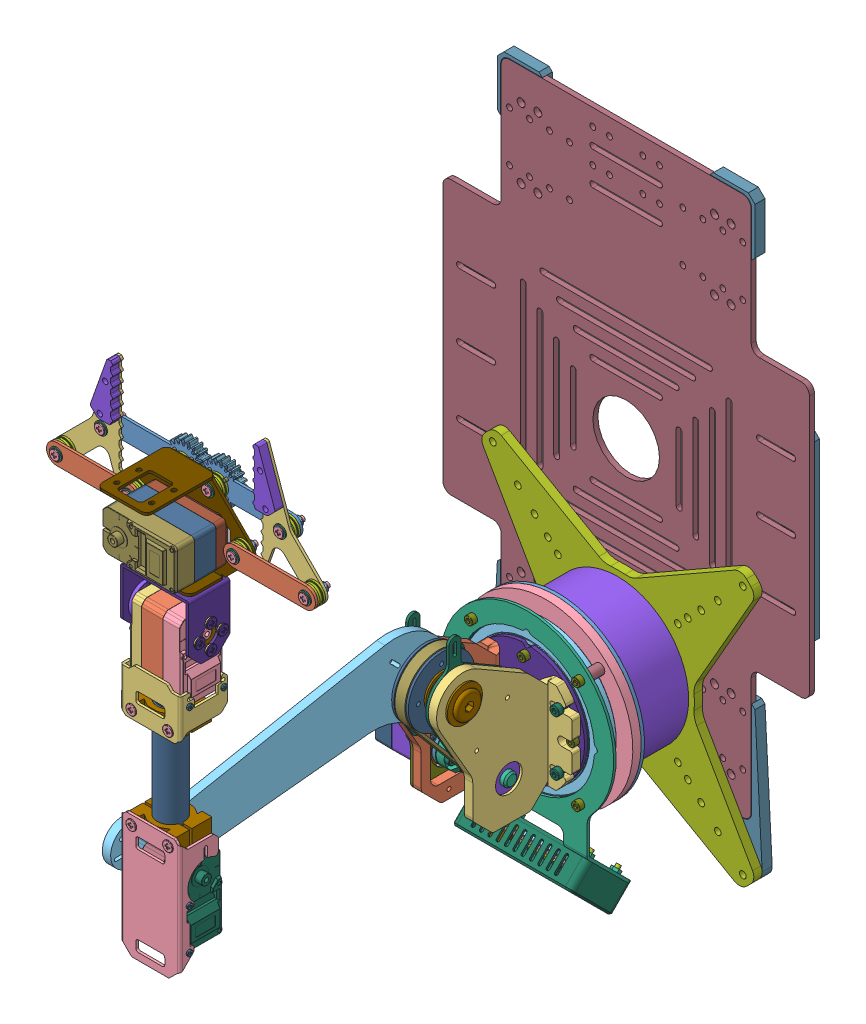
SolidWorks assembly RoArm-M1 STEP, configuration Default. Lengths in mm. (continued)
Components (placement in the parent): (continued)
- RoArm-M1 STEP(2)^RoArm-M1 STEP-1: RoArm-M1 STEP(2)^RoArm-M1 STEP [Default] at origin size (176.32 372.07 316.7) (virtual) (continued)
  - Servo Driver with ESP32^RoArm-M1 STEP(2)_RoArm-M1 STEP-1: Servo Driver with ESP32^RoArm-M1 STEP(2)_RoArm-M1 STEP [Default] at (-32.5 -89.0448 39.0323) x (1 0 0) z (0 -0.707107 0.707107) size (65.89 30.51 11.2) (virtual) (continued)
    - R20^Servo Driver with ESP32_RoArm-M1 STEP(2)_RoArm-M1 STEP-1: R20^Servo Driver with ESP32_RoArm-M1 STEP(2)_RoArm-M1 STEP [Default] at origin size (0.85 1.65 0.46) (virtual) (continued)
      - 490325136_1^R20_Servo Driver with ESP32_RoArm-M1 STEP(2)_RoArm-M1 STEP-1: 490325136_1^R20_Servo Driver with ESP32_RoArm-M1 STEP(2)_RoArm-M1 STEP [Default] at (15.5421 12.4002 0.025) size (0.8 1.5 0.42) (virtual)
        - Extruded (3)^490325136_1_R20_Servo Driver with ESP32_RoArm-M1 STEP(2)_RoArm-M1 STEP-1: Extruded (3)^490325136_1_R20_Servo Driver with ESP32_RoArm-M1 STEP(2)_RoArm-M1 STEP [Default] at origin size (0.8 1.5 0.42) (virtual)
    - L3(2)^Servo Driver with ESP32_RoArm-M1 STEP(2)_RoArm-M1 STEP-1: L3(2)^Servo Driver with ESP32_RoArm-M1 STEP(2)_RoArm-M1 STEP [Default] at origin size (4.4 4 1.97) (virtual)
      - 731907664^L3(2)_Servo Driver with ESP32_RoArm-M1 STEP(2)_RoArm-M1 STEP-1: 731907664^L3(2)_Servo Driver with ESP32_RoArm-M1 STEP(2)_RoArm-M1 STEP [Default] at (20.2 10.7008 0.025) size (4.4 4 1.97) (virtual)
        - Extruded (8)^731907664_L3(2)_Servo Driver with ESP32_RoArm-M1 STEP(2)_RoArm-M1 STEP-1: Extruded (8)^731907664_L3(2)_Servo Driver with ESP32_RoArm-M1 STEP(2)_RoArm-M1 STEP [Default] at origin size (4.4 4 1.97) (virtual)
    - C21^Servo Driver with ESP32_RoArm-M1 STEP(2)_RoArm-M1 STEP-1: C21^Servo Driver with ESP32_RoArm-M1 STEP(2)_RoArm-M1 STEP [Default] at origin size (1.65 0.85 0.46) (virtual)
      - 490324624_8^C21_Servo Driver with ESP32_RoArm-M1 STEP(2)_RoArm-M1 STEP-1: 490324624_8^C21_Servo Driver with ESP32_RoArm-M1 STEP(2)_RoArm-M1 STEP [Default] at (20.7358 7.4501 0.001) size (0.28 0.85 0.46) (virtual)
        - Extruded (6)^490324624_8_C21_Servo Driver with ESP32_RoArm-M1 STEP(2)_RoArm-M1 STEP-1: Extruded (6)^490324624_8_C21_Servo Driver with ESP32_RoArm-M1 STEP(2)_RoArm-M1 STEP [Default] at origin size (0.28 0.85 0.46) (virtual)
      - 490324624_9^C21_Servo Driver with ESP32_RoArm-M1 STEP(2)_RoArm-M1 STEP-1: 490324624_9^C21_Servo Driver with ESP32_RoArm-M1 STEP(2)_RoArm-M1 STEP [Default] at (19.3643 7.4501 0.001) size (0.28 0.85 0.46) (virtual)
        - Extruded (6)^490324624_9_C21_Servo Driver with ESP32_RoArm-M1 STEP(2)_RoArm-M1 STEP-1: Extruded (6)^490324624_9_C21_Servo Driver with ESP32_RoArm-M1 STEP(2)_RoArm-M1 STEP [Default] at origin size (0.28 0.85 0.46) (virtual)
      - 490324752_4^C21_Servo Driver with ESP32_RoArm-M1 STEP(2)_RoArm-M1 STEP-1: 490324752_4^C21_Servo Driver with ESP32_RoArm-M1 STEP(2)_RoArm-M1 STEP [Default] at (20.0501 7.4501 0.025) size (1.5 0.8 0.42) (virtual)
        - Extruded (7)^490324752_4_C21_Servo Driver with ESP32_RoArm-M1 STEP(2)_RoArm-M1 STEP-1: Extruded (7)^490324752_4_C21_Servo Driver with ESP32_RoArm-M1 STEP(2)_RoArm-M1 STEP [Default] at origin size (1.5 0.8 0.42) (virtual)
    - C20^Servo Driver with ESP32_RoArm-M1 STEP(2)_RoArm-M1 STEP-1: C20^Servo Driver with ESP32_RoArm-M1 STEP(2)_RoArm-M1 STEP [Default] at origin size (2.72 1.27 0.46) (virtual)
      - 490327952^C20_Servo Driver with ESP32_RoArm-M1 STEP(2)_RoArm-M1 STEP-1: 490327952^C20_Servo Driver with ESP32_RoArm-M1 STEP(2)_RoArm-M1 STEP [Default] at (19.6389 7.2746 -0.8615) size (2.29 1.12 0.42) (virtual)
        - Extruded (9)^490327952_C20_Servo Driver with ESP32_RoArm-M1 STEP(2)_RoArm-M1 STEP-1: Extruded (9)^490327952_C20_Servo Driver with ESP32_RoArm-M1 STEP(2)_RoArm-M1 STEP [Default] at origin size (2.29 1.12 0.42) (virtual)
      - 490327824^C20_Servo Driver with ESP32_RoArm-M1 STEP(2)_RoArm-M1 STEP-1: 490327824^C20_Servo Driver with ESP32_RoArm-M1 STEP(2)_RoArm-M1 STEP [Default] at (20.9194 7.2746 -0.8715) size (0.28 1.27 0.46) (virtual)
        - Extruded (10)^490327824_C20_Servo Driver with ESP32_RoArm-M1 STEP(2)_RoArm-M1 STEP-1: Extruded (10)^490327824_C20_Servo Driver with ESP32_RoArm-M1 STEP(2)_RoArm-M1 STEP [Default] at origin size (0.28 1.27 0.46) (virtual)
      - 490327824_1^C20_Servo Driver with ESP32_RoArm-M1 STEP(2)_RoArm-M1 STEP-1: 490327824_1^C20_Servo Driver with ESP32_RoArm-M1 STEP(2)_RoArm-M1 STEP [Default] at (18.4705 7.2746 -0.8715) size (0.28 1.27 0.46) (virtual)
        - Extruded (10)^490327824_1_C20_Servo Driver with ESP32_RoArm-M1 STEP(2)_RoArm-M1 STEP-1: Extruded (10)^490327824_1_C20_Servo Driver with ESP32_RoArm-M1 STEP(2)_RoArm-M1 STEP [Default] at origin size (0.28 1.27 0.46) (virtual)
    - C19^Servo Driver with ESP32_RoArm-M1 STEP(2)_RoArm-M1 STEP-1: C19^Servo Driver with ESP32_RoArm-M1 STEP(2)_RoArm-M1 STEP [Default] at origin size (1.65 0.85 0.46) (virtual)
      - 490324624_10^C19_Servo Driver with ESP32_RoArm-M1 STEP(2)_RoArm-M1 STEP-1: 490324624_10^C19_Servo Driver with ESP32_RoArm-M1 STEP(2)_RoArm-M1 STEP [Default] at (15.7063 7.4501 0.001) size (0.28 0.85 0.46) (virtual)
        - Extruded (6)^490324624_10_C19_Servo Driver with ESP32_RoArm-M1 STEP(2)_RoArm-M1 STEP-1: Extruded (6)^490324624_10_C19_Servo Driver with ESP32_RoArm-M1 STEP(2)_RoArm-M1 STEP [Default] at origin size (0.28 0.85 0.46) (virtual)
      - 490324624_11^C19_Servo Driver with ESP32_RoArm-M1 STEP(2)_RoArm-M1 STEP-1: 490324624_11^C19_Servo Driver with ESP32_RoArm-M1 STEP(2)_RoArm-M1 STEP [Default] at (17.0779 7.4501 0.001) size (0.28 0.85 0.46) (virtual)
        - Extruded (6)^490324624_11_C19_Servo Driver with ESP32_RoArm-M1 STEP(2)_RoArm-M1 STEP-1: Extruded (6)^490324624_11_C19_Servo Driver with ESP32_RoArm-M1 STEP(2)_RoArm-M1 STEP [Default] at origin size (0.28 0.85 0.46) (virtual)
      - 490324752_5^C19_Servo Driver with ESP32_RoArm-M1 STEP(2)_RoArm-M1 STEP-1: 490324752_5^C19_Servo Driver with ESP32_RoArm-M1 STEP(2)_RoArm-M1 STEP [Default] at (16.392 7.4501 0.025) size (1.5 0.8 0.42) (virtual)
        - Extruded (7)^490324752_5_C19_Servo Driver with ESP32_RoArm-M1 STEP(2)_RoArm-M1 STEP-1: Extruded (7)^490324752_5_C19_Servo Driver with ESP32_RoArm-M1 STEP(2)_RoArm-M1 STEP [Default] at origin size (1.5 0.8 0.42) (virtual)
    - C18^Servo Driver with ESP32_RoArm-M1 STEP(2)_RoArm-M1 STEP-1: C18^Servo Driver with ESP32_RoArm-M1 STEP(2)_RoArm-M1 STEP [Default] at origin size (1.65 0.85 0.46) (virtual)
      - 490324624_12^C18_Servo Driver with ESP32_RoArm-M1 STEP(2)_RoArm-M1 STEP-1: 490324624_12^C18_Servo Driver with ESP32_RoArm-M1 STEP(2)_RoArm-M1 STEP [Default] at (13.928 7.4503 0.001) size (0.28 0.85 0.46) (virtual)
        - Extruded (6)^490324624_12_C18_Servo Driver with ESP32_RoArm-M1 STEP(2)_RoArm-M1 STEP-1: Extruded (6)^490324624_12_C18_Servo Driver with ESP32_RoArm-M1 STEP(2)_RoArm-M1 STEP [Default] at origin size (0.28 0.85 0.46) (virtual)
      - 490324624_13^C18_Servo Driver with ESP32_RoArm-M1 STEP(2)_RoArm-M1 STEP-1: 490324624_13^C18_Servo Driver with ESP32_RoArm-M1 STEP(2)_RoArm-M1 STEP [Default] at (12.5564 7.4503 0.001) size (0.28 0.85 0.46) (virtual)
        - Extruded (6)^490324624_13_C18_Servo Driver with ESP32_RoArm-M1 STEP(2)_RoArm-M1 STEP-1: Extruded (6)^490324624_13_C18_Servo Driver with ESP32_RoArm-M1 STEP(2)_RoArm-M1 STEP [Default] at origin size (0.28 0.85 0.46) (virtual)
      - 490324752_6^C18_Servo Driver with ESP32_RoArm-M1 STEP(2)_RoArm-M1 STEP-1: 490324752_6^C18_Servo Driver with ESP32_RoArm-M1 STEP(2)_RoArm-M1 STEP [Default] at (13.2423 7.4503 0.025) size (1.5 0.8 0.42) (virtual)
        - Extruded (7)^490324752_6_C18_Servo Driver with ESP32_RoArm-M1 STEP(2)_RoArm-M1 STEP-1: Extruded (7)^490324752_6_C18_Servo Driver with ESP32_RoArm-M1 STEP(2)_RoArm-M1 STEP [Default] at origin size (1.5 0.8 0.42) (virtual)
    - C17^Servo Driver with ESP32_RoArm-M1 STEP(2)_RoArm-M1 STEP-1: C17^Servo Driver with ESP32_RoArm-M1 STEP(2)_RoArm-M1 STEP [Default] at origin size (2.72 1.27 0.46) (virtual)
      - 490327952_1^C17_Servo Driver with ESP32_RoArm-M1 STEP(2)_RoArm-M1 STEP-1: 490327952_1^C17_Servo Driver with ESP32_RoArm-M1 STEP(2)_RoArm-M1 STEP [Default] at (8.4889 7.2746 -0.8615) size (2.29 1.12 0.42) (virtual)
        - Extruded (9)^490327952_1_C17_Servo Driver with ESP32_RoArm-M1 STEP(2)_RoArm-M1 STEP-1: Extruded (9)^490327952_1_C17_Servo Driver with ESP32_RoArm-M1 STEP(2)_RoArm-M1 STEP [Default] at origin size (2.29 1.12 0.42) (virtual)
      - 490327824_2^C17_Servo Driver with ESP32_RoArm-M1 STEP(2)_RoArm-M1 STEP-1: 490327824_2^C17_Servo Driver with ESP32_RoArm-M1 STEP(2)_RoArm-M1 STEP [Default] at (9.7694 7.2746 -0.8715) size (0.28 1.27 0.46) (virtual)
        - Extruded (10)^490327824_2_C17_Servo Driver with ESP32_RoArm-M1 STEP(2)_RoArm-M1 STEP-1: Extruded (10)^490327824_2_C17_Servo Driver with ESP32_RoArm-M1 STEP(2)_RoArm-M1 STEP [Default] at origin size (0.28 1.27 0.46) (virtual)
      - 490327824_3^C17_Servo Driver with ESP32_RoArm-M1 STEP(2)_RoArm-M1 STEP-1: 490327824_3^C17_Servo Driver with ESP32_RoArm-M1 STEP(2)_RoArm-M1 STEP [Default] at (7.3205 7.2746 -0.8715) size (0.28 1.27 0.46) (virtual)
        - Extruded (10)^490327824_3_C17_Servo Driver with ESP32_RoArm-M1 STEP(2)_RoArm-M1 STEP-1: Extruded (10)^490327824_3_C17_Servo Driver with ESP32_RoArm-M1 STEP(2)_RoArm-M1 STEP [Default] at origin size (0.28 1.27 0.46) (virtual)
    - C16^Servo Driver with ESP32_RoArm-M1 STEP(2)_RoArm-M1 STEP-1: C16^Servo Driver with ESP32_RoArm-M1 STEP(2)_RoArm-M1 STEP [Default] at origin size (0.85 1.65 0.46) (virtual)
      - 490325008_4^C16_Servo Driver with ESP32_RoArm-M1 STEP(2)_RoArm-M1 STEP-1: 490325008_4^C16_Servo Driver with ESP32_RoArm-M1 STEP(2)_RoArm-M1 STEP [Default] at (17.042 13.0861 0.001) size (0.85 0.28 0.46) (virtual)
        - Extruded (2)^490325008_4_C16_Servo Driver with ESP32_RoArm-M1 STEP(2)_RoArm-M1 STEP-1: Extruded (2)^490325008_4_C16_Servo Driver with ESP32_RoArm-M1 STEP(2)_RoArm-M1 STEP [Default] at origin size (0.85 0.28 0.46) (virtual)
      - 490325008_5^C16_Servo Driver with ESP32_RoArm-M1 STEP(2)_RoArm-M1 STEP-1: 490325008_5^C16_Servo Driver with ESP32_RoArm-M1 STEP(2)_RoArm-M1 STEP [Default] at (17.042 11.7146 0.001) size (0.85 0.28 0.46) (virtual)
        - Extruded (2)^490325008_5_C16_Servo Driver with ESP32_RoArm-M1 STEP(2)_RoArm-M1 STEP-1: Extruded (2)^490325008_5_C16_Servo Driver with ESP32_RoArm-M1 STEP(2)_RoArm-M1 STEP [Default] at origin size (0.85 0.28 0.46) (virtual)
      - 490325136_2^C16_Servo Driver with ESP32_RoArm-M1 STEP(2)_RoArm-M1 STEP-1: 490325136_2^C16_Servo Driver with ESP32_RoArm-M1 STEP(2)_RoArm-M1 STEP [Default] at (17.042 12.4004 0.025) size (0.8 1.5 0.42) (virtual)
        - Extruded (3)^490325136_2_C16_Servo Driver with ESP32_RoArm-M1 STEP(2)_RoArm-M1 STEP-1: Extruded (3)^490325136_2_C16_Servo Driver with ESP32_RoArm-M1 STEP(2)_RoArm-M1 STEP [Default] at origin size (0.8 1.5 0.42) (virtual)
    - C14^Servo Driver with ESP32_RoArm-M1 STEP(2)_RoArm-M1 STEP-1: C14^Servo Driver with ESP32_RoArm-M1 STEP(2)_RoArm-M1 STEP [Default] at origin size (1.65 0.85 0.46) (virtual)
      - 490324624_14^C14_Servo Driver with ESP32_RoArm-M1 STEP(2)_RoArm-M1 STEP-1: 490324624_14^C14_Servo Driver with ESP32_RoArm-M1 STEP(2)_RoArm-M1 STEP [Default] at (54.614 11.7078 0.001) size (0.28 0.85 0.46) (virtual)
        - Extruded (6)^490324624_14_C14_Servo Driver with ESP32_RoArm-M1 STEP(2)_RoArm-M1 STEP-1: Extruded (6)^490324624_14_C14_Servo Driver with ESP32_RoArm-M1 STEP(2)_RoArm-M1 STEP [Default] at origin size (0.28 0.85 0.46) (virtual)
      - 490324624_15^C14_Servo Driver with ESP32_RoArm-M1 STEP(2)_RoArm-M1 STEP-1: 490324624_15^C14_Servo Driver with ESP32_RoArm-M1 STEP(2)_RoArm-M1 STEP [Default] at (55.9855 11.7078 0.001) size (0.28 0.85 0.46) (virtual)
        - Extruded (6)^490324624_15_C14_Servo Driver with ESP32_RoArm-M1 STEP(2)_RoArm-M1 STEP-1: Extruded (6)^490324624_15_C14_Servo Driver with ESP32_RoArm-M1 STEP(2)_RoArm-M1 STEP [Default] at origin size (0.28 0.85 0.46) (virtual)
      - 490324752_7^C14_Servo Driver with ESP32_RoArm-M1 STEP(2)_RoArm-M1 STEP-1: 490324752_7^C14_Servo Driver with ESP32_RoArm-M1 STEP(2)_RoArm-M1 STEP [Default] at (55.2997 11.7078 0.025) size (1.5 0.8 0.42) (virtual)
        - Extruded (7)^490324752_7_C14_Servo Driver with ESP32_RoArm-M1 STEP(2)_RoArm-M1 STEP-1: Extruded (7)^490324752_7_C14_Servo Driver with ESP32_RoArm-M1 STEP(2)_RoArm-M1 STEP [Default] at origin size (1.5 0.8 0.42) (virtual)
    - R16^Servo Driver with ESP32_RoArm-M1 STEP(2)_RoArm-M1 STEP-1: R16^Servo Driver with ESP32_RoArm-M1 STEP(2)_RoArm-M1 STEP [Default] at origin size (1.65 0.85 0.46) (virtual)
      - 490324624_16^R16_Servo Driver with ESP32_RoArm-M1 STEP(2)_RoArm-M1 STEP-1: 490324624_16^R16_Servo Driver with ESP32_RoArm-M1 STEP(2)_RoArm-M1 STEP [Default] at (52.2655 21.0579 -0.8715) size (0.28 0.85 0.46) (virtual)
        - Extruded (6)^490324624_16_R16_Servo Driver with ESP32_RoArm-M1 STEP(2)_RoArm-M1 STEP-1: Extruded (6)^490324624_16_R16_Servo Driver with ESP32_RoArm-M1 STEP(2)_RoArm-M1 STEP [Default] at origin size (0.28 0.85 0.46) (virtual)
      - 490324624_17^R16_Servo Driver with ESP32_RoArm-M1 STEP(2)_RoArm-M1 STEP-1: 490324624_17^R16_Servo Driver with ESP32_RoArm-M1 STEP(2)_RoArm-M1 STEP [Default] at (53.637 21.0579 -0.8715) size (0.28 0.85 0.46) (virtual)
        - Extruded (6)^490324624_17_R16_Servo Driver with ESP32_RoArm-M1 STEP(2)_RoArm-M1 STEP-1: Extruded (6)^490324624_17_R16_Servo Driver with ESP32_RoArm-M1 STEP(2)_RoArm-M1 STEP [Default] at origin size (0.28 0.85 0.46) (virtual)
      - 490324752_8^R16_Servo Driver with ESP32_RoArm-M1 STEP(2)_RoArm-M1 STEP-1: 490324752_8^R16_Servo Driver with ESP32_RoArm-M1 STEP(2)_RoArm-M1 STEP [Default] at (52.9512 21.0579 -0.8615) size (1.5 0.8 0.42) (virtual)
        - Extruded (7)^490324752_8_R16_Servo Driver with ESP32_RoArm-M1 STEP(2)_RoArm-M1 STEP-1: Extruded (7)^490324752_8_R16_Servo Driver with ESP32_RoArm-M1 STEP(2)_RoArm-M1 STEP [Default] at origin size (1.5 0.8 0.42) (virtual)
    - R3^Servo Driver with ESP32_RoArm-M1 STEP(2)_RoArm-M1 STEP-1: R3^Servo Driver with ESP32_RoArm-M1 STEP(2)_RoArm-M1 STEP [Default] at origin size (0.85 1.65 0.46) (virtual)
      - 490325008_6^R3_Servo Driver with ESP32_RoArm-M1 STEP(2)_RoArm-M1 STEP-1: 490325008_6^R3_Servo Driver with ESP32_RoArm-M1 STEP(2)_RoArm-M1 STEP [Default] at (25.6497 14.2437 0.001) size (0.85 0.28 0.46) (virtual)
        - Extruded (2)^490325008_6_R3_Servo Driver with ESP32_RoArm-M1 STEP(2)_RoArm-M1 STEP-1: Extruded (2)^490325008_6_R3_Servo Driver with ESP32_RoArm-M1 STEP(2)_RoArm-M1 STEP [Default] at origin size (0.85 0.28 0.46) (virtual)
      - 490325008_7^R3_Servo Driver with ESP32_RoArm-M1 STEP(2)_RoArm-M1 STEP-1: 490325008_7^R3_Servo Driver with ESP32_RoArm-M1 STEP(2)_RoArm-M1 STEP [Default] at (25.6497 12.8721 0.001) size (0.85 0.28 0.46) (virtual)
        - Extruded (2)^490325008_7_R3_Servo Driver with ESP32_RoArm-M1 STEP(2)_RoArm-M1 STEP-1: Extruded (2)^490325008_7_R3_Servo Driver with ESP32_RoArm-M1 STEP(2)_RoArm-M1 STEP [Default] at origin size (0.85 0.28 0.46) (virtual)
      - 490325136_3^R3_Servo Driver with ESP32_RoArm-M1 STEP(2)_RoArm-M1 STEP-1: 490325136_3^R3_Servo Driver with ESP32_RoArm-M1 STEP(2)_RoArm-M1 STEP [Default] at (25.6497 13.558 0.025) size (0.8 1.5 0.42) (virtual)
        - Extruded (3)^490325136_3_R3_Servo Driver with ESP32_RoArm-M1 STEP(2)_RoArm-M1 STEP-1: Extruded (3)^490325136_3_R3_Servo Driver with ESP32_RoArm-M1 STEP(2)_RoArm-M1 STEP [Default] at origin size (0.8 1.5 0.42) (virtual)
    - D2^Servo Driver with ESP32_RoArm-M1 STEP(2)_RoArm-M1 STEP-1: D2^Servo Driver with ESP32_RoArm-M1 STEP(2)_RoArm-M1 STEP [Default] at origin size (2.7 1.5 1.2) (virtual)
      - 731906512^D2_Servo Driver with ESP32_RoArm-M1 STEP(2)_RoArm-M1 STEP-1: 731906512^D2_Servo Driver with ESP32_RoArm-M1 STEP(2)_RoArm-M1 STEP [Default] at (53.8498 17.7079 -0.6655) size (0.8 0.4 0.25) (virtual)
        - Extruded (11)^731906512_D2_Servo Driver with ESP32_RoArm-M1 STEP(2)_RoArm-M1 STEP-1: Extruded (11)^731906512_D2_Servo Driver with ESP32_RoArm-M1 STEP(2)_RoArm-M1 STEP [Default] at origin size (0.8 0.4 0.25) (virtual)
      - 731906384^D2_Servo Driver with ESP32_RoArm-M1 STEP(2)_RoArm-M1 STEP-1: 731906384^D2_Servo Driver with ESP32_RoArm-M1 STEP(2)_RoArm-M1 STEP [Default] at (52.8998 17.7079 -1.6115) size (2 1.5 1.18) (virtual)
        - Extruded (12)^731906384_D2_Servo Driver with ESP32_RoArm-M1 STEP(2)_RoArm-M1 STEP-1: Extruded (12)^731906384_D2_Servo Driver with ESP32_RoArm-M1 STEP(2)_RoArm-M1 STEP [Default] at origin size (2 1.5 1.18) (virtual)
      - 731906512_1^D2_Servo Driver with ESP32_RoArm-M1 STEP(2)_RoArm-M1 STEP-1: 731906512_1^D2_Servo Driver with ESP32_RoArm-M1 STEP(2)_RoArm-M1 STEP [Default] at (51.9498 17.7079 -0.6655) size (0.8 0.4 0.25) (virtual)
        - Extruded (11)^731906512_1_D2_Servo Driver with ESP32_RoArm-M1 STEP(2)_RoArm-M1 STEP-1: Extruded (11)^731906512_1_D2_Servo Driver with ESP32_RoArm-M1 STEP(2)_RoArm-M1 STEP [Default] at origin size (0.8 0.4 0.25) (virtual)
    - R19^Servo Driver with ESP32_RoArm-M1 STEP(2)_RoArm-M1 STEP-1: R19^Servo Driver with ESP32_RoArm-M1 STEP(2)_RoArm-M1 STEP [Default] at origin size (1.65 0.85 0.46) (virtual)
      - 490324624_18^R19_Servo Driver with ESP32_RoArm-M1 STEP(2)_RoArm-M1 STEP-1: 490324624_18^R19_Servo Driver with ESP32_RoArm-M1 STEP(2)_RoArm-M1 STEP [Default] at (52.2655 15.9079 -0.8715) size (0.28 0.85 0.46) (virtual)
        - Extruded (6)^490324624_18_R19_Servo Driver with ESP32_RoArm-M1 STEP(2)_RoArm-M1 STEP-1: Extruded (6)^490324624_18_R19_Servo Driver with ESP32_RoArm-M1 STEP(2)_RoArm-M1 STEP [Default] at origin size (0.28 0.85 0.46) (virtual)
      - 490324624_19^R19_Servo Driver with ESP32_RoArm-M1 STEP(2)_RoArm-M1 STEP-1: 490324624_19^R19_Servo Driver with ESP32_RoArm-M1 STEP(2)_RoArm-M1 STEP [Default] at (53.637 15.9079 -0.8715) size (0.28 0.85 0.46) (virtual)
        - Extruded (6)^490324624_19_R19_Servo Driver with ESP32_RoArm-M1 STEP(2)_RoArm-M1 STEP-1: Extruded (6)^490324624_19_R19_Servo Driver with ESP32_RoArm-M1 STEP(2)_RoArm-M1 STEP [Default] at origin size (0.28 0.85 0.46) (virtual)
      - 490324752_9^R19_Servo Driver with ESP32_RoArm-M1 STEP(2)_RoArm-M1 STEP-1: 490324752_9^R19_Servo Driver with ESP32_RoArm-M1 STEP(2)_RoArm-M1 STEP [Default] at (52.9512 15.9079 -0.8615) size (1.5 0.8 0.42) (virtual)
        - Extruded (7)^490324752_9_R19_Servo Driver with ESP32_RoArm-M1 STEP(2)_RoArm-M1 STEP-1: Extruded (7)^490324752_9_R19_Servo Driver with ESP32_RoArm-M1 STEP(2)_RoArm-M1 STEP [Default] at origin size (1.5 0.8 0.42) (virtual)
    - R18^Servo Driver with ESP32_RoArm-M1 STEP(2)_RoArm-M1 STEP-1: R18^Servo Driver with ESP32_RoArm-M1 STEP(2)_RoArm-M1 STEP [Default] at origin size (1.65 0.85 0.46) (virtual)
      - 490324624_20^R18_Servo Driver with ESP32_RoArm-M1 STEP(2)_RoArm-M1 STEP-1: 490324624_20^R18_Servo Driver with ESP32_RoArm-M1 STEP(2)_RoArm-M1 STEP [Default] at (52.2655 23.9579 -0.8715) size (0.28 0.85 0.46) (virtual)
        - Extruded (6)^490324624_20_R18_Servo Driver with ESP32_RoArm-M1 STEP(2)_RoArm-M1 STEP-1: Extruded (6)^490324624_20_R18_Servo Driver with ESP32_RoArm-M1 STEP(2)_RoArm-M1 STEP [Default] at origin size (0.28 0.85 0.46) (virtual)
      - 490324624_21^R18_Servo Driver with ESP32_RoArm-M1 STEP(2)_RoArm-M1 STEP-1: 490324624_21^R18_Servo Driver with ESP32_RoArm-M1 STEP(2)_RoArm-M1 STEP [Default] at (53.637 23.9579 -0.8715) size (0.28 0.85 0.46) (virtual)
        - Extruded (6)^490324624_21_R18_Servo Driver with ESP32_RoArm-M1 STEP(2)_RoArm-M1 STEP-1: Extruded (6)^490324624_21_R18_Servo Driver with ESP32_RoArm-M1 STEP(2)_RoArm-M1 STEP [Default] at origin size (0.28 0.85 0.46) (virtual)
      - 490324752_10^R18_Servo Driver with ESP32_RoArm-M1 STEP(2)_RoArm-M1 STEP-1: 490324752_10^R18_Servo Driver with ESP32_RoArm-M1 STEP(2)_RoArm-M1 STEP [Default] at (52.9512 23.9579 -0.8615) size (1.5 0.8 0.42) (virtual)
        - Extruded (7)^490324752_10_R18_Servo Driver with ESP32_RoArm-M1 STEP(2)_RoArm-M1 STEP-1: Extruded (7)^490324752_10_R18_Servo Driver with ESP32_RoArm-M1 STEP(2)_RoArm-M1 STEP [Default] at origin size (1.5 0.8 0.42) (virtual)
    - C11^Servo Driver with ESP32_RoArm-M1 STEP(2)_RoArm-M1 STEP-1: C11^Servo Driver with ESP32_RoArm-M1 STEP(2)_RoArm-M1 STEP [Default] at origin size (1.65 0.85 0.46) (virtual)
      - 490324624_22^C11_Servo Driver with ESP32_RoArm-M1 STEP(2)_RoArm-M1 STEP-1: 490324624_22^C11_Servo Driver with ESP32_RoArm-M1 STEP(2)_RoArm-M1 STEP [Default] at (52.2655 28.3079 -0.8715) size (0.28 0.85 0.46) (virtual)
        - Extruded (6)^490324624_22_C11_Servo Driver with ESP32_RoArm-M1 STEP(2)_RoArm-M1 STEP-1: Extruded (6)^490324624_22_C11_Servo Driver with ESP32_RoArm-M1 STEP(2)_RoArm-M1 STEP [Default] at origin size (0.28 0.85 0.46) (virtual)
      - 490324624_23^C11_Servo Driver with ESP32_RoArm-M1 STEP(2)_RoArm-M1 STEP-1: 490324624_23^C11_Servo Driver with ESP32_RoArm-M1 STEP(2)_RoArm-M1 STEP [Default] at (53.637 28.3079 -0.8715) size (0.28 0.85 0.46) (virtual)
        - Extruded (6)^490324624_23_C11_Servo Driver with ESP32_RoArm-M1 STEP(2)_RoArm-M1 STEP-1: Extruded (6)^490324624_23_C11_Servo Driver with ESP32_RoArm-M1 STEP(2)_RoArm-M1 STEP [Default] at origin size (0.28 0.85 0.46) (virtual)
      - 490324752_11^C11_Servo Driver with ESP32_RoArm-M1 STEP(2)_RoArm-M1 STEP-1: 490324752_11^C11_Servo Driver with ESP32_RoArm-M1 STEP(2)_RoArm-M1 STEP [Default] at (52.9512 28.3079 -0.8615) size (1.5 0.8 0.42) (virtual)
        - Extruded (7)^490324752_11_C11_Servo Driver with ESP32_RoArm-M1 STEP(2)_RoArm-M1 STEP-1: Extruded (7)^490324752_11_C11_Servo Driver with ESP32_RoArm-M1 STEP(2)_RoArm-M1 STEP [Default] at origin size (1.5 0.8 0.42) (virtual)
    - C10^Servo Driver with ESP32_RoArm-M1 STEP(2)_RoArm-M1 STEP-1: C10^Servo Driver with ESP32_RoArm-M1 STEP(2)_RoArm-M1 STEP [Default] at origin size (1.65 0.85 0.46) (virtual)
      - 490324624_24^C10_Servo Driver with ESP32_RoArm-M1 STEP(2)_RoArm-M1 STEP-1: 490324624_24^C10_Servo Driver with ESP32_RoArm-M1 STEP(2)_RoArm-M1 STEP [Default] at (52.2655 26.8579 -0.8715) size (0.28 0.85 0.46) (virtual)
        - Extruded (6)^490324624_24_C10_Servo Driver with ESP32_RoArm-M1 STEP(2)_RoArm-M1 STEP-1: Extruded (6)^490324624_24_C10_Servo Driver with ESP32_RoArm-M1 STEP(2)_RoArm-M1 STEP [Default] at origin size (0.28 0.85 0.46) (virtual)
      - 490324624_25^C10_Servo Driver with ESP32_RoArm-M1 STEP(2)_RoArm-M1 STEP-1: 490324624_25^C10_Servo Driver with ESP32_RoArm-M1 STEP(2)_RoArm-M1 STEP [Default] at (53.637 26.8579 -0.8715) size (0.28 0.85 0.46) (virtual)
        - Extruded (6)^490324624_25_C10_Servo Driver with ESP32_RoArm-M1 STEP(2)_RoArm-M1 STEP-1: Extruded (6)^490324624_25_C10_Servo Driver with ESP32_RoArm-M1 STEP(2)_RoArm-M1 STEP [Default] at origin size (0.28 0.85 0.46) (virtual)
      - 490324752_12^C10_Servo Driver with ESP32_RoArm-M1 STEP(2)_RoArm-M1 STEP-1: 490324752_12^C10_Servo Driver with ESP32_RoArm-M1 STEP(2)_RoArm-M1 STEP [Default] at (52.9512 26.8579 -0.8615) size (1.5 0.8 0.42) (virtual)
        - Extruded (7)^490324752_12_C10_Servo Driver with ESP32_RoArm-M1 STEP(2)_RoArm-M1 STEP-1: Extruded (7)^490324752_12_C10_Servo Driver with ESP32_RoArm-M1 STEP(2)_RoArm-M1 STEP [Default] at origin size (1.5 0.8 0.42) (virtual)
    - C9^Servo Driver with ESP32_RoArm-M1 STEP(2)_RoArm-M1 STEP-1: C9^Servo Driver with ESP32_RoArm-M1 STEP(2)_RoArm-M1 STEP [Default] at origin size (1.65 0.85 0.46) (virtual)
      - 490324624_26^C9_Servo Driver with ESP32_RoArm-M1 STEP(2)_RoArm-M1 STEP-1: 490324624_26^C9_Servo Driver with ESP32_RoArm-M1 STEP(2)_RoArm-M1 STEP [Default] at (52.2655 25.4079 -0.8715) size (0.28 0.85 0.46) (virtual)
        - Extruded (6)^490324624_26_C9_Servo Driver with ESP32_RoArm-M1 STEP(2)_RoArm-M1 STEP-1: Extruded (6)^490324624_26_C9_Servo Driver with ESP32_RoArm-M1 STEP(2)_RoArm-M1 STEP [Default] at origin size (0.28 0.85 0.46) (virtual)
      - 490324624_27^C9_Servo Driver with ESP32_RoArm-M1 STEP(2)_RoArm-M1 STEP-1: 490324624_27^C9_Servo Driver with ESP32_RoArm-M1 STEP(2)_RoArm-M1 STEP [Default] at (53.637 25.4079 -0.8715) size (0.28 0.85 0.46) (virtual)
        - Extruded (6)^490324624_27_C9_Servo Driver with ESP32_RoArm-M1 STEP(2)_RoArm-M1 STEP-1: Extruded (6)^490324624_27_C9_Servo Driver with ESP32_RoArm-M1 STEP(2)_RoArm-M1 STEP [Default] at origin size (0.28 0.85 0.46) (virtual)
      - 490324752_13^C9_Servo Driver with ESP32_RoArm-M1 STEP(2)_RoArm-M1 STEP-1: 490324752_13^C9_Servo Driver with ESP32_RoArm-M1 STEP(2)_RoArm-M1 STEP [Default] at (52.9512 25.4079 -0.8615) size (1.5 0.8 0.42) (virtual)
        - Extruded (7)^490324752_13_C9_Servo Driver with ESP32_RoArm-M1 STEP(2)_RoArm-M1 STEP-1: Extruded (7)^490324752_13_C9_Servo Driver with ESP32_RoArm-M1 STEP(2)_RoArm-M1 STEP [Default] at origin size (1.5 0.8 0.42) (virtual)
    - C8^Servo Driver with ESP32_RoArm-M1 STEP(2)_RoArm-M1 STEP-1: C8^Servo Driver with ESP32_RoArm-M1 STEP(2)_RoArm-M1 STEP [Default] at origin size (1.65 0.85 0.46) (virtual)
      - 490324624_28^C8_Servo Driver with ESP32_RoArm-M1 STEP(2)_RoArm-M1 STEP-1: 490324624_28^C8_Servo Driver with ESP32_RoArm-M1 STEP(2)_RoArm-M1 STEP [Default] at (51.9153 15.1578 0.001) size (0.28 0.85 0.46) (virtual)
        - Extruded (6)^490324624_28_C8_Servo Driver with ESP32_RoArm-M1 STEP(2)_RoArm-M1 STEP-1: Extruded (6)^490324624_28_C8_Servo Driver with ESP32_RoArm-M1 STEP(2)_RoArm-M1 STEP [Default] at origin size (0.28 0.85 0.46) (virtual)
      - 490324624_29^C8_Servo Driver with ESP32_RoArm-M1 STEP(2)_RoArm-M1 STEP-1: 490324624_29^C8_Servo Driver with ESP32_RoArm-M1 STEP(2)_RoArm-M1 STEP [Default] at (53.2868 15.1578 0.001) size (0.28 0.85 0.46) (virtual)
        - Extruded (6)^490324624_29_C8_Servo Driver with ESP32_RoArm-M1 STEP(2)_RoArm-M1 STEP-1: Extruded (6)^490324624_29_C8_Servo Driver with ESP32_RoArm-M1 STEP(2)_RoArm-M1 STEP [Default] at origin size (0.28 0.85 0.46) (virtual)
      - 490324752_14^C8_Servo Driver with ESP32_RoArm-M1 STEP(2)_RoArm-M1 STEP-1: 490324752_14^C8_Servo Driver with ESP32_RoArm-M1 STEP(2)_RoArm-M1 STEP [Default] at (52.601 15.1578 0.025) size (1.5 0.8 0.42) (virtual)
        - Extruded (7)^490324752_14_C8_Servo Driver with ESP32_RoArm-M1 STEP(2)_RoArm-M1 STEP-1: Extruded (7)^490324752_14_C8_Servo Driver with ESP32_RoArm-M1 STEP(2)_RoArm-M1 STEP [Default] at origin size (1.5 0.8 0.42) (virtual)
    - C7^Servo Driver with ESP32_RoArm-M1 STEP(2)_RoArm-M1 STEP-1: C7^Servo Driver with ESP32_RoArm-M1 STEP(2)_RoArm-M1 STEP [Default] at origin size (1.65 0.85 0.46) (virtual)
      - 490324624_30^C7_Servo Driver with ESP32_RoArm-M1 STEP(2)_RoArm-M1 STEP-1: 490324624_30^C7_Servo Driver with ESP32_RoArm-M1 STEP(2)_RoArm-M1 STEP [Default] at (48.6639 15.1578 0.001) size (0.28 0.85 0.46) (virtual)
        - Extruded (6)^490324624_30_C7_Servo Driver with ESP32_RoArm-M1 STEP(2)_RoArm-M1 STEP-1: Extruded (6)^490324624_30_C7_Servo Driver with ESP32_RoArm-M1 STEP(2)_RoArm-M1 STEP [Default] at origin size (0.28 0.85 0.46) (virtual)
      - 490324624_31^C7_Servo Driver with ESP32_RoArm-M1 STEP(2)_RoArm-M1 STEP-1: 490324624_31^C7_Servo Driver with ESP32_RoArm-M1 STEP(2)_RoArm-M1 STEP [Default] at (50.0355 15.1578 0.001) size (0.28 0.85 0.46) (virtual)
        - Extruded (6)^490324624_31_C7_Servo Driver with ESP32_RoArm-M1 STEP(2)_RoArm-M1 STEP-1: Extruded (6)^490324624_31_C7_Servo Driver with ESP32_RoArm-M1 STEP(2)_RoArm-M1 STEP [Default] at origin size (0.28 0.85 0.46) (virtual)
      - 490324752_15^C7_Servo Driver with ESP32_RoArm-M1 STEP(2)_RoArm-M1 STEP-1: 490324752_15^C7_Servo Driver with ESP32_RoArm-M1 STEP(2)_RoArm-M1 STEP [Default] at (49.3497 15.1578 0.025) size (1.5 0.8 0.42) (virtual)
        - Extruded (7)^490324752_15_C7_Servo Driver with ESP32_RoArm-M1 STEP(2)_RoArm-M1 STEP-1: Extruded (7)^490324752_15_C7_Servo Driver with ESP32_RoArm-M1 STEP(2)_RoArm-M1 STEP [Default] at origin size (1.5 0.8 0.42) (virtual)
    - VT2^Servo Driver with ESP32_RoArm-M1 STEP(2)_RoArm-M1 STEP-1: VT2^Servo Driver with ESP32_RoArm-M1 STEP(2)_RoArm-M1 STEP [Default] at origin size (3.58 2.9 0.55) (virtual)
      - 513870512^VT2_Servo Driver with ESP32_RoArm-M1 STEP(2)_RoArm-M1 STEP-1: 513870512^VT2_Servo Driver with ESP32_RoArm-M1 STEP(2)_RoArm-M1 STEP [Default] at (29.962 9.9054 0) size (1.17 0.58 0.16) (virtual)
        - Extruded (13)^513870512_VT2_Servo Driver with ESP32_RoArm-M1 STEP(2)_RoArm-M1 STEP-1: Extruded (13)^513870512_VT2_Servo Driver with ESP32_RoArm-M1 STEP(2)_RoArm-M1 STEP [Default] at origin size (1.17 0.58 0.16) (virtual)
      - 682612656^VT2_Servo Driver with ESP32_RoArm-M1 STEP(2)_RoArm-M1 STEP-1: 682612656^VT2_Servo Driver with ESP32_RoArm-M1 STEP(2)_RoArm-M1 STEP [Default] at (28.7498 9.9079 0.045) size (1.3 2.9 0.5) (virtual)
        - Extruded (14)^682612656_VT2_Servo Driver with ESP32_RoArm-M1 STEP(2)_RoArm-M1 STEP-1: Extruded (14)^682612656_VT2_Servo Driver with ESP32_RoArm-M1 STEP(2)_RoArm-M1 STEP [Default] at origin size (1.3 2.9 0.5) (virtual)
      - 513870512_1^VT2_Servo Driver with ESP32_RoArm-M1 STEP(2)_RoArm-M1 STEP-1: 513870512_1^VT2_Servo Driver with ESP32_RoArm-M1 STEP(2)_RoArm-M1 STEP [Default] at (27.549 10.8706 0) size (1.17 0.58 0.16) (virtual)
        - Extruded (13)^513870512_1_VT2_Servo Driver with ESP32_RoArm-M1 STEP(2)_RoArm-M1 STEP-1: Extruded (13)^513870512_1_VT2_Servo Driver with ESP32_RoArm-M1 STEP(2)_RoArm-M1 STEP [Default] at origin size (1.17 0.58 0.16) (virtual)
      - 513870512_2^VT2_Servo Driver with ESP32_RoArm-M1 STEP(2)_RoArm-M1 STEP-1: 513870512_2^VT2_Servo Driver with ESP32_RoArm-M1 STEP(2)_RoArm-M1 STEP [Default] at (27.549 8.9402 0) size (1.17 0.58 0.16) (virtual)
        - Extruded (13)^513870512_2_VT2_Servo Driver with ESP32_RoArm-M1 STEP(2)_RoArm-M1 STEP-1: Extruded (13)^513870512_2_VT2_Servo Driver with ESP32_RoArm-M1 STEP(2)_RoArm-M1 STEP [Default] at origin size (1.17 0.58 0.16) (virtual)
    - VT1^Servo Driver with ESP32_RoArm-M1 STEP(2)_RoArm-M1 STEP-1: VT1^Servo Driver with ESP32_RoArm-M1 STEP(2)_RoArm-M1 STEP [Default] at origin size (3.58 2.9 0.55) (virtual)
      - 513870512_3^VT1_Servo Driver with ESP32_RoArm-M1 STEP(2)_RoArm-M1 STEP-1: 513870512_3^VT1_Servo Driver with ESP32_RoArm-M1 STEP(2)_RoArm-M1 STEP [Default] at (29.9938 13.4822 0) size (1.17 0.58 0.16) (virtual)
        - Extruded (13)^513870512_3_VT1_Servo Driver with ESP32_RoArm-M1 STEP(2)_RoArm-M1 STEP-1: Extruded (13)^513870512_3_VT1_Servo Driver with ESP32_RoArm-M1 STEP(2)_RoArm-M1 STEP [Default] at origin size (1.17 0.58 0.16) (virtual)
      - 682612656_1^VT1_Servo Driver with ESP32_RoArm-M1 STEP(2)_RoArm-M1 STEP-1: 682612656_1^VT1_Servo Driver with ESP32_RoArm-M1 STEP(2)_RoArm-M1 STEP [Default] at (28.7816 13.4847 0.045) size (1.3 2.9 0.5) (virtual)
        - Extruded (14)^682612656_1_VT1_Servo Driver with ESP32_RoArm-M1 STEP(2)_RoArm-M1 STEP-1: Extruded (14)^682612656_1_VT1_Servo Driver with ESP32_RoArm-M1 STEP(2)_RoArm-M1 STEP [Default] at origin size (1.3 2.9 0.5) (virtual)
      - 513870512_4^VT1_Servo Driver with ESP32_RoArm-M1 STEP(2)_RoArm-M1 STEP-1: 513870512_4^VT1_Servo Driver with ESP32_RoArm-M1 STEP(2)_RoArm-M1 STEP [Default] at (27.5808 14.4474 0) size (1.17 0.58 0.16) (virtual)
        - Extruded (13)^513870512_4_VT1_Servo Driver with ESP32_RoArm-M1 STEP(2)_RoArm-M1 STEP-1: Extruded (13)^513870512_4_VT1_Servo Driver with ESP32_RoArm-M1 STEP(2)_RoArm-M1 STEP [Default] at origin size (1.17 0.58 0.16) (virtual)
      - 513870512_5^VT1_Servo Driver with ESP32_RoArm-M1 STEP(2)_RoArm-M1 STEP-1: 513870512_5^VT1_Servo Driver with ESP32_RoArm-M1 STEP(2)_RoArm-M1 STEP [Default] at (27.5808 12.517 0) size (1.17 0.58 0.16) (virtual)
        - Extruded (13)^513870512_5_VT1_Servo Driver with ESP32_RoArm-M1 STEP(2)_RoArm-M1 STEP-1: Extruded (13)^513870512_5_VT1_Servo Driver with ESP32_RoArm-M1 STEP(2)_RoArm-M1 STEP [Default] at origin size (1.17 0.58 0.16) (virtual)
    - U2^Servo Driver with ESP32_RoArm-M1 STEP(2)_RoArm-M1 STEP-1: U2^Servo Driver with ESP32_RoArm-M1 STEP(2)_RoArm-M1 STEP [Default] at origin size (32 11.5 1.42) (virtual)
      - User_Library-0_91___OLED_v4^U2_Servo Driver with ESP32_RoArm-M1 STEP(2)_RoArm-M1 STEP-1: User_Library-0_91___OLED_v4^U2_Servo Driver with ESP32_RoArm-M1 STEP(2)_RoArm-M1 STEP [Default] at (24.7497 28.2578 0) x (1 0 0) z (0 -1 0) size (32 1.42 11.5) (virtual)
    - S2^Servo Driver with ESP32_RoArm-M1 STEP(2)_RoArm-M1 STEP-1: S2^Servo Driver with ESP32_RoArm-M1 STEP(2)_RoArm-M1 STEP [Default] at origin size (4.5 3.1 2.55) (virtual)
      - SMT_Tactile_Switch_PTS-820^S2_Servo Driver with ESP32_RoArm-M1 STEP(2)_RoArm-M1 STEP-1: SMT_Tactile_Switch_PTS-820^S2_Servo Driver with ESP32_RoArm-M1 STEP(2)_RoArm-M1 STEP [Default] at (61.7997 8.3578 0) x (-1 0 0) z (0 1 0) size (4.5 2.55 3.1) (virtual)
    - S1^Servo Driver with ESP32_RoArm-M1 STEP(2)_RoArm-M1 STEP-1: S1^Servo Driver with ESP32_RoArm-M1 STEP(2)_RoArm-M1 STEP [Default] at origin size (4.5 3.1 2.55) (virtual)
      - SMT_Tactile_Switch_PTS-820^S1_Servo Driver with ESP32_RoArm-M1 STEP(2)_RoArm-M1 STEP-1: SMT_Tactile_Switch_PTS-820^S1_Servo Driver with ESP32_RoArm-M1 STEP(2)_RoArm-M1 STEP [Default] at (61.7997 21.6578 0) x (-1 0 0) z (0 1 0) size (4.5 2.55 3.1) (virtual)
    - R15^Servo Driver with ESP32_RoArm-M1 STEP(2)_RoArm-M1 STEP-1: R15^Servo Driver with ESP32_RoArm-M1 STEP(2)_RoArm-M1 STEP [Default] at origin size (0.85 1.65 0.46) (virtual)
      - 490325008_8^R15_Servo Driver with ESP32_RoArm-M1 STEP(2)_RoArm-M1 STEP-1: 490325008_8^R15_Servo Driver with ESP32_RoArm-M1 STEP(2)_RoArm-M1 STEP [Default] at (17.7499 20.9937 -0.8715) size (0.85 0.28 0.46) (virtual)
        - Extruded (2)^490325008_8_R15_Servo Driver with ESP32_RoArm-M1 STEP(2)_RoArm-M1 STEP-1: Extruded (2)^490325008_8_R15_Servo Driver with ESP32_RoArm-M1 STEP(2)_RoArm-M1 STEP [Default] at origin size (0.85 0.28 0.46) (virtual)
      - 490325008_9^R15_Servo Driver with ESP32_RoArm-M1 STEP(2)_RoArm-M1 STEP-1: 490325008_9^R15_Servo Driver with ESP32_RoArm-M1 STEP(2)_RoArm-M1 STEP [Default] at (17.7499 19.6221 -0.8715) size (0.85 0.28 0.46) (virtual)
        - Extruded (2)^490325008_9_R15_Servo Driver with ESP32_RoArm-M1 STEP(2)_RoArm-M1 STEP-1: Extruded (2)^490325008_9_R15_Servo Driver with ESP32_RoArm-M1 STEP(2)_RoArm-M1 STEP [Default] at origin size (0.85 0.28 0.46) (virtual)
      - 490325136_4^R15_Servo Driver with ESP32_RoArm-M1 STEP(2)_RoArm-M1 STEP-1: 490325136_4^R15_Servo Driver with ESP32_RoArm-M1 STEP(2)_RoArm-M1 STEP [Default] at (17.7499 20.308 -0.8615) size (0.8 1.5 0.42) (virtual)
        - Extruded (3)^490325136_4_R15_Servo Driver with ESP32_RoArm-M1 STEP(2)_RoArm-M1 STEP-1: Extruded (3)^490325136_4_R15_Servo Driver with ESP32_RoArm-M1 STEP(2)_RoArm-M1 STEP [Default] at origin size (0.8 1.5 0.42) (virtual)
    - R14^Servo Driver with ESP32_RoArm-M1 STEP(2)_RoArm-M1 STEP-1: R14^Servo Driver with ESP32_RoArm-M1 STEP(2)_RoArm-M1 STEP [Default] at origin size (0.85 1.65 0.46) (virtual)
